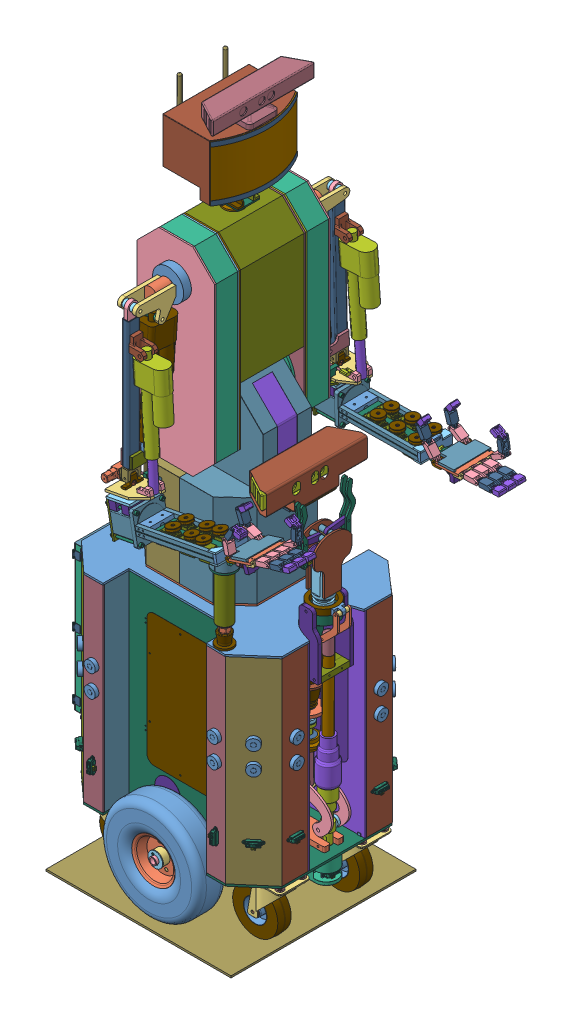
SolidWorks assembly sorbot, configuration По умолчанию. Lengths in mm. (continued)
Mates (geometry in assembly coordinates): (continued)
- Совпадение572: coincident anti-aligned: plane of HS-311 Hitec Standard Servo and Horn-3/HS-311-p2-1 through (120.3857 893.7008 114.0983) normal (-0.185706 0.982605 0); plane of lower.arm.p9-2 through (118.2362 893.2946 122.4974) normal (0.185706 -0.982605 0)
- Совпадение573: coincident anti-aligned: plane of HS-311 Hitec Standard Servo and Horn-2/HS-311-p2-1 through (174.429 903.9147 111.5983) normal (-0.185706 0.982605 0); plane of lower.arm.p9-5 through (172.2795 903.5084 119.9974) normal (0.185706 -0.982605 0)
- Совпадение574: coincident anti-aligned: plane of HS-311 Hitec Standard Servo and Horn-4/HS-311-p2-1 through (203.8531 909.4756 125.8336) normal (-0.185706 0.982605 0); plane of lower.arm.p9-6 through (206.0025 909.8819 117.4346) normal (0.185706 -0.982605 0)
- Заблокировать245: lock: unknown of ?; unknown of lower.arm.p9-4
- Заблокировать246: lock: unknown of ?; unknown of lower.arm.p9-3
- Заблокировать247: lock: unknown of ?; unknown of lower.arm.p9-6
- Заблокировать248: lock: unknown of ?; unknown of lower.arm.p9-5
- Заблокировать249: lock: unknown of ?; unknown of lower.arm.p9-2
- Заблокировать250: lock: unknown of lower.arm.p2-1; unknown of lower.arm.p8-2
- Совпадение582: coincident anti-aligned: plane of palm.p1-3 through (364.9952 940.9838 91.5947) normal (0.311571 -0.950223 0); plane of palm.p3-1 through (346.841 935.0312 91.3484) normal (-0.311571 0.950223 0)
- Совпадение583: coincident anti-aligned: plane of palm.p1-3 through (361.9011 946.2836 191.5864) normal (0.950144 0.311545 0.012888); plane of palm.p3-1 through (362.0352 950.0109 91.5947) normal (-0.950144 -0.311545 -0.012888)
- Совпадение584: coincident aligned: plane of palm.p1-3 through (290.6402 922.9177 190.6197) normal (-0.012247 -0.004016 0.999917); plane of palm.p3-1 through (369.3773 952.4183 191.7026) normal (-0.012247 -0.004016 0.999917)
- Заблокировать261: lock: unknown of lower.arm.p8-2; unknown of palm.fixture.p4-4
- Заблокировать262: lock: unknown of lower.arm.p8-2; unknown of palm.fixture.p4-1
- Заблокировать265: lock: unknown of lower.arm.p8-2; unknown of palm.fixture.p4-3
- Заблокировать266: lock: unknown of lower.arm.p8-2; unknown of palm.fixture.p4-5
- Концентричный332: concentric aligned: cylinder of palm.p3-1 through (367.5649 947.6145 91.6528) axis (-0.012247 -0.004016 0.999917) radius 1.5; cylinder of finger.p1-1 through (366.6096 947.3013 169.6463) axis (-0.012247 -0.004016 0.999917) radius 1.5
- Концентричный333: concentric anti-aligned: cylinder of finger.p1-1 through (366.6096 947.3013 169.6463) axis (-0.012247 -0.004016 0.999917) radius 1.5; cylinder of finger.spring-1 through (366.5011 947.2657 178.5056) axis (0.012247 0.004016 -0.999917) radius 1.9307
- Касательный23: tangent anti-aligned: plane of finger.p1-1 through (351.8589 937.2027 182.1761) normal (0.012247 0.004016 -0.999917); cylinder of finger.spring-1 through (357.2133 941.7472 181.9199) axis (0.950144 0.311545 0.012888) radius 0.34
- Параллельность161: parallel aligned: plane of finger.p1-1 through (363.4168 940.9924 169.5819) normal (-0.950144 -0.311545 -0.012888); plane of finger.spring-1 through (357.2133 941.7472 181.9199) normal (-0.950144 -0.311545 -0.012888)
- Концентричный334: concentric aligned: cylinder of palm.p3-1 through (367.5649 947.6145 91.6528) axis (-0.012247 -0.004016 0.999917) radius 1.5; cylinder of palm.fixture.p13-1 through (367.5656 947.6147 91.5963) axis (-0.012247 -0.004016 0.999917) radius 1.5
- Совпадение627: coincident anti-aligned: plane of palm.p3-1 through (362.243 935.8718 186.5483) normal (0.012247 0.004016 -0.999917); plane of finger.p1-1 through (357.4065 939.0217 186.5017) normal (-0.012247 -0.004016 0.999917)
- Параллельность160: parallel aligned: plane of palm.p1-3 through (363.1257 946.6851 91.5947) normal (-0.311571 0.950223 0); plane of finger.p1-1 through (406.9341 967.89 190.7246) normal (-0.311571 0.950223 0)
- Концентричный339: concentric aligned: cylinder of palm.fixture.p13-1 through (367.5656 947.6147 91.5963) axis (-0.012247 -0.004016 0.999917) radius 1.5; cylinder of finger.p1-2 through (367.5465 947.6085 93.1527) axis (-0.012247 -0.004016 0.999917) radius 1.5
- Концентричный342: concentric aligned: cylinder of palm.fixture.p13-1 through (367.5656 947.6147 91.5963) axis (-0.012247 -0.004016 0.999917) radius 1.5; cylinder of finger.p1-3 through (366.9219 947.4037 144.1484) axis (-0.012247 -0.004016 0.999917) radius 1.5
- Параллельность165: parallel aligned: plane of palm.p1-3 through (363.1257 946.6851 91.5947) normal (-0.311571 0.950223 0); plane of finger.p1-3 through (407.2464 967.9924 165.2267) normal (-0.311571 0.950223 0)
- Совпадение637: coincident anti-aligned: plane of palm.p1-3 through (364.9952 940.9838 91.5947) normal (0.311571 -0.950223 0); plane of palm.p3.m-1 through (323.3155 927.3173 191.0376) normal (-0.311571 0.950223 0)
- Совпадение638: coincident aligned: plane of palm.p1-3 through (290.6402 922.9177 190.6197) normal (-0.012247 -0.004016 0.999917); plane of palm.p3.m-1 through (290.9518 925.1246 190.6324) normal (-0.012247 -0.004016 0.999917)
- Совпадение640: coincident anti-aligned: plane of palm.p3.m-1 through (299.2015 928.9006 190.7486) normal (0.950144 0.311545 0.012888); plane of palm.p1-3 through (300.4356 926.1295 166.7506) normal (-0.950144 -0.311545 -0.012888)
- Совпадение641: coincident anti-aligned: plane of palm.p3-1 through (363.3452 936.2333 96.5558) normal (-0.012247 -0.004016 0.999917); plane of finger.p1-2 through (360.8495 937.3933 96.5299) normal (0.012247 0.004016 -0.999917)
- Концентричный345: concentric aligned: cylinder of palm.fixture.p13-1 through (367.5656 947.6147 91.5963) axis (-0.012247 -0.004016 0.999917) radius 1.5; cylinder of finger.p1-4 through (367.2342 947.5061 118.6505) axis (-0.012247 -0.004016 0.999917) radius 1.5
- Параллельность167: parallel aligned: plane of palm.p1-3 through (363.1257 946.6851 91.5947) normal (-0.311571 0.950223 0); plane of finger.p1-4 through (407.5587 968.0948 139.7288) normal (-0.311571 0.950223 0)
- Совпадение645: coincident anti-aligned: plane of palm.p1-3 through (364.9952 940.9838 91.5947) normal (0.311571 -0.950223 0); plane of palm.p3.m-2 through (324.2768 927.6326 112.5441) normal (-0.311571 0.950223 0)
- Совпадение646: coincident aligned: plane of palm.p1-3 through (291.8649 923.3193 90.628) normal (0.012247 0.004016 -0.999917); plane of palm.p3.m-2 through (292.1765 925.5262 90.6407) normal (0.012247 0.004016 -0.999917)
- Совпадение647: coincident anti-aligned: plane of palm.p3.m-2 through (300.1629 929.2158 112.2551) normal (0.950144 0.311545 0.012888); plane of palm.p1-3 through (301.0725 926.3383 114.7549) normal (-0.950144 -0.311545 -0.012888)
- Заблокировать267: lock: unknown of palm.p3-1; unknown of palm.fixture.p13-1
- Концентричный348: concentric aligned: cylinder of palm.p3.m-1 through (296.5509 922.5164 190.6905) axis (0.012247 0.004016 -0.999917) radius 1.5; cylinder of finger.p1-5 through (296.557 922.5184 190.1906) axis (0.012247 0.004016 -0.999917) radius 1.5
- Совпадение648: coincident anti-aligned: plane of palm.p3.m-1 through (289.0079 911.8586 186.555) normal (0.012247 0.004016 -0.999917); plane of finger.p1-5 through (294.0033 910.6326 186.6113) normal (-0.012247 -0.004016 0.999917)
- Концентричный351: concentric aligned: cylinder of finger.p1-6 through (297.5172 922.8332 111.7971) axis (0.012247 0.004016 -0.999917) radius 1.5; cylinder of palm.p3.m-2 through (297.5123 922.8316 112.197) axis (0.012247 0.004016 -0.999917) radius 1.5
- Концентричный352: concentric aligned: cylinder of finger.p1-1 through (405.2463 959.4437 170.1683) axis (-0.012247 -0.004016 0.999917) radius 1.5; cylinder of finger.p2-7 through (405.2463 959.4437 170.1683) axis (-0.012247 -0.004016 0.999917) radius 1.5
- Совпадение652: coincident anti-aligned: plane of finger.p1-1 through (399.3202 952.7649 186.5702) normal (0.012247 0.004016 -0.999917); plane of finger.p2-7 through (396.174 952.0257 186.5287) normal (-0.012247 -0.004016 0.999917)
- Концентричный354: concentric: cylinder of finger.p3-1 through (466.5916 802.6812 273.0909) axis (-0.001318 0.191299 0.981531) radius 1.5; cylinder of finger.p2-7 through (466.5917 802.6596 272.9801) axis (-0.001318 0.191299 0.981531) radius 1.5
- Совпадение653: coincident: plane of finger.p3-1 through (235.2448 521.1837 179.8569) normal (0.004463 0.000114 0.99999); plane of finger.p2-7 through (237.0318 518.7761 179.8492) normal (-0.004463 -0.000114 -0.99999)
- Концентричный355: concentric aligned: cylinder of finger.p1-3 through (405.5586 959.5461 144.6704) axis (-0.012247 -0.004016 0.999917) radius 1.5; cylinder of finger.p2-8 through (405.5586 959.5461 144.6704) axis (-0.012247 -0.004016 0.999917) radius 1.5
- Совпадение654: coincident anti-aligned: plane of finger.p1-3 through (399.6325 952.8673 161.0724) normal (0.012247 0.004016 -0.999917); plane of finger.p2-8 through (396.6473 951.938 161.0321) normal (-0.012247 -0.004016 0.999917)
- Концентричный356: concentric aligned: cylinder of finger.p1-4 through (405.8709 959.6485 119.1725) axis (-0.012247 -0.004016 0.999917) radius 1.5; cylinder of finger.p2-9 through (405.8709 959.6485 119.1725) axis (-0.012247 -0.004016 0.999917) radius 1.5
- Совпадение655: coincident anti-aligned: plane of finger.p1-4 through (399.9448 952.9697 135.5745) normal (0.012247 0.004016 -0.999917); plane of finger.p2-9 through (396.9974 951.997 135.5345) normal (-0.012247 -0.004016 0.999917)
- Концентричный357: concentric aligned: cylinder of finger.p1-2 through (401.9154 969.0333 93.6596) axis (-0.012247 -0.004016 0.999917) radius 1.5; cylinder of finger.p2-10 through (401.9154 969.0333 93.6596) axis (-0.012247 -0.004016 0.999917) radius 1.5
- Совпадение656: coincident anti-aligned: plane of finger.p1-2 through (397.826 961.1324 110.0792) normal (0.012247 0.004016 -0.999917); plane of finger.p2-10 through (406.346 958.4178 110.1726) normal (-0.012247 -0.004016 0.999917)
- Концентричный358: concentric aligned: cylinder of finger.p3-2 through (401.4238 1008.0295 93.9231) axis (-0.012247 -0.004016 0.999917) radius 1.5; cylinder of finger.p2-10 through (401.4252 1008.0299 93.8102) axis (-0.012247 -0.004016 0.999917) radius 1.5
- Совпадение657: coincident anti-aligned: plane of finger.p3-2 through (412.7357 1007.5295 110.4481) normal (-0.012247 -0.004016 0.999917); plane of finger.p2-10 through (405.8167 1000.5207 110.3352) normal (0.012247 0.004016 -0.999917)
- Концентричный359: concentric aligned: cylinder of finger.p1-5 through (287.6988 962.0409 190.2408) axis (0.012247 0.004016 -0.999917) radius 1.5; cylinder of finger.p2-11 through (287.6988 962.0409 190.2408) axis (0.012247 0.004016 -0.999917) radius 1.5
- Совпадение658: coincident anti-aligned: plane of finger.p1-5 through (284.8951 953.7891 186.173) normal (0.012247 0.004016 -0.999917); plane of finger.p2-11 through (278.3955 955.3292 186.0996) normal (-0.012247 -0.004016 0.999917)
- Концентричный360: concentric aligned: cylinder of finger.p3-5 through (307.9454 995.3702 190.7355) axis (0.012247 0.004016 -0.999917) radius 1.5; cylinder of finger.p2-11 through (307.9467 995.3707 190.6226) axis (0.012247 0.004016 -0.999917) radius 1.5
- Совпадение659: coincident anti-aligned: plane of finger.p3-5 through (298.337 1001.6675 186.5299) normal (-0.012247 -0.004016 0.999917); plane of finger.p2-11 through (300.2563 991.3138 186.5118) normal (0.012247 0.004016 -0.999917)
- Концентричный362: concentric aligned: cylinder of finger.p1-6 through (259.3107 936.2716 111.3831) axis (0.012247 0.004016 -0.999917) radius 1.5; cylinder of finger.p2-12 through (259.3107 936.2716 111.3831) axis (0.012247 0.004016 -0.999917) radius 1.5
- Совпадение661: coincident anti-aligned: plane of finger.p1-6 through (264.8581 929.4858 107.4234) normal (0.012247 0.004016 -0.999917); plane of finger.p2-12 through (259.1122 924.7688 107.3341) normal (-0.012247 -0.004016 0.999917)
- Концентричный363: concentric aligned: cylinder of finger.p3-6 through (195.7839 707.1121 106.7239) axis (-0.004463 -0.000114 -0.99999) radius 1.5; cylinder of finger.p2-12 through (195.7834 707.1121 106.6111) axis (-0.004463 -0.000114 -0.99999) radius 1.5
- Совпадение662: coincident: plane of finger.p3-6 through (190.3026 717.2558 102.6343) normal (0.004463 0.000114 0.99999); plane of finger.p2-12 through (187.0589 706.2794 102.6501) normal (-0.004463 -0.000114 -0.99999)
- Совпадение664: coincident anti-aligned: plane of palm.p3-1 through (373.957 939.7128 161.2051) normal (0.012247 0.004016 -0.999917); plane of finger.p1-3 through (357.7188 939.1241 161.0039) normal (-0.012247 -0.004016 0.999917)
- Совпадение665: coincident anti-aligned: plane of palm.p3-1 through (374.2693 939.8152 135.7072) normal (0.012247 0.004016 -0.999917); plane of finger.p1-4 through (358.0311 939.2265 135.506) normal (-0.012247 -0.004016 0.999917)
- Совпадение666: coincident anti-aligned: plane of palm.p1-3 through (363.1257 946.6851 91.5947) normal (-0.311571 0.950223 0); plane of palm.p5-1 through (330.6828 936.0474 170.4076) normal (0.311571 -0.950223 0)
- Совпадение667: coincident anti-aligned: plane of palm.p1-3 through (363.1257 946.6851 91.5947) normal (-0.311571 0.950223 0); plane of palm.p6-1 through (301.0674 926.3367 156.6492) normal (0.311571 -0.950223 0)
- Совпадение668: coincident anti-aligned: plane of palm.p1-3 through (363.1257 946.6851 91.5947) normal (-0.311571 0.950223 0); plane of palm.p5-2 through (331.3758 936.2746 112.4456) normal (0.311571 -0.950223 0)
- Совпадение669: coincident anti-aligned: plane of palm.p1-3 through (363.1257 946.6851 91.5947) normal (-0.311571 0.950223 0); plane of palm.p6-2 through (301.386 926.4412 124.555) normal (0.311571 -0.950223 0)
- Заблокировать268: lock: unknown of palm.p1-3; unknown of palm.cap-1
- Совпадение692: coincident anti-aligned: plane of arm.p1.m-1 through (-3.763 964.7884 152.9102) normal (1 0 0); plane of forearm.rotate.p12-m-1 through (-3.763 985.2277 154.0338) normal (-1 0 0)
- Параллельность178: parallel aligned: plane of forearm.rotate.p12-m-1 through (-3.763 964.7884 154.0338) normal (0 0 1); plane of arm.p1.m-1 through (-18.263 964.7884 156.4102) normal (0 0 1)
- Заблокировать282: lock: unknown of arm.p1.m-1; unknown of forearm.rotate.p12-m-1
- Концентричный381: concentric aligned: cylinder of finger.p3-3 through (442.6662 971.5314 145.2986) axis (-0.012247 -0.004016 0.999917) radius 1.5; cylinder of finger.p2-8 through (442.6677 971.5319 145.173) axis (-0.012247 -0.004016 0.999917) radius 1.5
- Концентричный382: concentric aligned: cylinder of finger.p3-4 through (442.9206 971.8199 119.5969) axis (-0.012247 -0.004016 0.999917) radius 1.5; cylinder of finger.p2-9 through (442.9196 971.8196 119.6752) axis (-0.012247 -0.004016 0.999917) radius 1.5
- Заблокировать287: lock: unknown of finger.p1-1; unknown of finger.spring-2
- Заблокировать288: lock: unknown of finger.p1-1; unknown of finger1.rod-1
- Заблокировать290: lock: unknown of palm.p1-3; unknown of finger.p1-1
- Заблокировать291: lock: unknown of finger.p1-1; unknown of finger.p2-7
- Заблокировать293: lock: unknown of palm.p1-3; unknown of finger.p1-3
- Заблокировать294: lock: unknown of finger.p1-3; unknown of finger.p2-8
- Заблокировать295: lock: unknown of finger.p3-3; unknown of finger.p2-8
- Заблокировать296: lock: unknown of finger.p1-4; unknown of finger.p2-9
- Заблокировать297: lock: unknown of finger.p3-4; unknown of finger.p2-9
- Заблокировать298: lock: unknown of palm.p1-3; unknown of finger.p1-2
- Заблокировать299: lock: unknown of finger.p1-2; unknown of finger.p2-10
- Заблокировать301: lock: unknown of palm.p1-3; unknown of finger.p1-5
- Заблокировать302: lock: unknown of finger.p1-5; unknown of finger.p2-11
- Заблокировать304: lock: unknown of finger.p3-5; unknown of finger.p2-11
- Заблокировать305: lock: unknown of finger.p1-6; unknown of finger.p2-12
- Заблокировать306: lock: unknown of finger.p3-6; unknown of finger.p2-12
- Заблокировать307: lock: unknown of palm.p1-3; unknown of palm.p6-2
- Заблокировать308: lock: unknown of palm.p1-3; unknown of palm.p6-1
- Заблокировать309: lock: unknown of palm.p1-3; unknown of palm.p5-2
- Заблокировать310: lock: unknown of palm.p1-3; unknown of palm.p5-1
- Заблокировать311: lock: unknown of palm.p1-3; unknown of palm.fixture.p14-1
- Заблокировать319: lock: unknown of palm.p3-1; unknown of palm.fixture.p13-1
- Концентричный386: concentric aligned: cylinder of body.frame.p1-3 through (-12.4559 1335.4922 -50.7442) axis (0 0 1) radius 43; cylinder of arm.fixture.cap-1 through (-12.4559 1335.4922 -73.2442) axis (0 0 1) radius 45
- Заблокировать330: lock: unknown of body_axis-1; unknown of body.frame.p1.fixture-1
- Заблокировать336: lock: unknown of body.frame.p2-1; unknown of body.frame.p1-3
- Заблокировать337: lock: unknown of body.frame.p2-1; unknown of body.frame.p3-1
- Совпадение740: coincident anti-aligned: plane of shoulder.bearing.housing-2 through (-12.4903 1335.516 -46.7442) normal (0 0 1); plane of body.frame.p4.right-1 through (-117.4903 1436.2936 -46.7442) normal (0 0 -1)
- Концентричный404: concentric aligned: cylinder of shoulder.bearing.housing-1 through (-12.7629 1335.3853 40.2558) axis (0 0 -1) radius 15.5; cylinder of shoulder.axis-1 through (-12.7629 1335.3853 44.2558) axis (0 0 -1) radius 15
- Совпадение742: coincident: unknown of shoulder.bearing.housing-2; unknown of shoulder.axis-1
- Заблокировать361: lock: unknown of shoulder.p6-1; unknown of shoulder.axis-1
- Заблокировать362: lock: unknown of shoulder.p6-2; unknown of shoulder.axis-1
- Совпадение745: coincident anti-aligned: plane of body.frame.p5-1 through (92.4017 957.5916 592.5032) normal (1 0 0); plane of cap-hinge-1 through (92.4017 1325.4557 -46.5922) normal (-1 0 0)
- Совпадение746: coincident anti-aligned: plane of body.frame.p5-1 through (92.4017 957.5916 592.5032) normal (1 0 0); plane of cap-hinge-p1-2 through (92.4017 1182.6154 -46.8053) normal (-1 0 0)
- Концентричный405: concentric anti-aligned: cylinder of cap-hinge-2 through (95.4017 1143.4534 -46.8053) axis (0 1 0) radius 2; cylinder of cap-hinge-p1-2 through (95.4017 1182.6154 -46.8053) axis (0 -1 0) radius 2
- Совпадение747: coincident anti-aligned: plane of cap-hinge-2 through (75.4017 1173.4534 -40.9717) normal (0 -1 0); plane of cap-hinge-p1-2 through (75.4017 1173.4534 -41.8622) normal (0 1 0)
- Заблокировать363: lock: unknown of body.frame.p5-1; unknown of cap-hinge-1
- Заблокировать364: lock: unknown of body.frame.p5-1; unknown of cap-hinge-p1-2
- Касательный31: tangent anti-aligned: cylinder of arm.actuator.p2-2 through (-12.7848 967.3083 102.1523) axis (0 0.997661 -0.068351) radius 10; plane of forearm.rotate.p12-1 through (-22.7848 999.7884 125.248) normal (1 0 0)
- Параллельность188: parallel anti-aligned: cylinder of arm.actuator-2/arm.actuator.p1-1 through (-27.7848 1286.6873 80.2712) axis (1 0 0) radius 4.1; cylinder of arm.actuator.p2-2 through (12.2152 975.7884 101.5713) axis (-1 0 0) radius 4
- Заблокировать368: lock: unknown of shoulder.axis-1; unknown of arm.fixture-2
- Заблокировать369: lock: unknown of arm.p1.m-1; unknown of shoulder.lever-1
- Совпадение765: coincident anti-aligned: plane of arm.p1.m-1 through (-18.263 964.7884 125.9102) normal (0 0 1); plane of shoulder.lever-1 through (-17.763 1335.3853 125.9102) normal (0 0 -1)
- Концентричный406: concentric anti-aligned: cylinder of arm.fixture-2 through (-27.7629 1335.3853 140.1602) axis (-1 0 0) radius 4; cylinder of shoulder.lever-1 through (-17.763 1335.3853 140.1602) axis (1 0 0) radius 4
- Концентричный408: concentric aligned: cylinder of arm.lift2.actuator.fixture.p1-1 through (-17.763 1335.3853 140.1602) axis (-1 0 0) radius 4; cylinder of arm.fixture-2 through (-27.7629 1335.3853 140.1602) axis (-1 0 0) radius 4
- Совпадение757: coincident anti-aligned: plane of shoulder.lever-1 through (-17.763 1335.3853 140.1608) normal (-1 0 0); plane of arm.lift2.actuator.fixture.p1-1 through (-17.763 1335.3853 140.1602) normal (1 0 0)
- Концентричный409: concentric anti-aligned: cylinder of arm.actuator-2/arm.actuator.p1-1 through (-27.7848 1286.6873 80.2712) axis (1 0 0) radius 4.1; cylinder of arm.fixture-2 through (-27.7629 1286.6873 80.2712) axis (-1 0 0) radius 4
- Совпадение759: coincident anti-aligned: plane of arm.fixture-2 through (-27.7629 1335.3734 139.2441) normal (1 0 0); plane of arm.lift2.actuator.fixture.p1.m1-1 through (-27.7629 1286.6873 80.2712) normal (-1 0 0)
- Концентричный411: concentric anti-aligned: cylinder of arm.actuator-2/arm.actuator.p1-1 through (-27.7848 1286.6873 80.2712) axis (1 0 0) radius 4.1; cylinder of arm.lift2.actuator.fixture.p1.m1-1 through (-22.7629 1286.6873 80.2712) axis (-1 0 0) radius 4
- Совпадение760: coincident anti-aligned: plane of shoulder.axis-1 through (2.2371 1356.1502 -67.7442) normal (1 0 0); plane of arm.fixture-3 through (2.2371 1335.3734 139.2441) normal (-1 0 0)
- Концентричный412: concentric anti-aligned: cylinder of shoulder.lever-1 through (-17.763 1335.3853 140.1602) axis (1 0 0) radius 4; cylinder of arm.fixture-3 through (12.2371 1335.3853 140.1602) axis (-1 0 0) radius 4
- Концентричный413: concentric aligned: cylinder of arm.fixture-3 through (12.2371 1335.3853 140.1602) axis (-1 0 0) radius 4; cylinder of arm.lift2.actuator.fixture.p1-3 through (2.2371 1335.3853 140.1602) axis (-1 0 0) radius 4
- Совпадение761: coincident anti-aligned: plane of arm.fixture-3 through (2.2371 1335.3734 139.2441) normal (-1 0 0); plane of arm.lift2.actuator.fixture.p1-3 through (2.2371 1335.3853 140.1602) normal (1 0 0)
- Концентричный414: concentric anti-aligned: cylinder of arm.actuator-2/arm.actuator.p1-1 through (-27.7848 1286.6873 80.2712) axis (1 0 0) radius 4.1; cylinder of arm.lift2.actuator.fixture.p1.m1-2 through (2.2371 1286.6873 80.2712) axis (-1 0 0) radius 4
- Совпадение762: coincident anti-aligned: plane of arm.fixture-3 through (2.2371 1335.3734 139.2441) normal (-1 0 0); plane of arm.lift2.actuator.fixture.p1.m1-2 through (2.2371 1286.6873 80.2712) normal (1 0 0)
- Концентричный416: concentric anti-aligned: cylinder of arm.actuator-2/arm.actuator.p1-1 through (-27.7848 1286.6873 80.2712) axis (1 0 0) radius 4.1; cylinder of arm.fixture-3 through (12.2371 1286.6873 80.2712) axis (-1 0 0) radius 4
- Заблокировать370: lock: unknown of shoulder.axis-1; unknown of arm.fixture-3
- Концентричный420: concentric aligned: cylinder of body.center-1 through (-20.0648 982.0246 -136.9555) axis (0 -1 0) radius 11; cylinder of body_pivot-2 through (-20.0648 982.0246 -136.9555) axis (0 -1 0) radius 11
- Заблокировать371: lock: unknown of body.center-1; unknown of body_pivot_fixture-1
- Совпадение768: coincident anti-aligned: plane of body_pivot_fixture-1 through (-20.0648 972.0246 -136.9555) normal (0 1 0); plane of body_pivot-2 through (-63.8424 972.0246 -151.4602) normal (0 -1 0)
- Заблокировать372: lock: unknown of body.frame.p2-1; unknown of cap-hinge-p1-1
- Концентричный421: concentric anti-aligned: cylinder of body_axis-1 through (-20.0648 1016.5246 -50.7475) axis (0 0 -1) radius 10.9; cylinder of body.tilt.axis.frame-2 through (-20.0648 1016.5246 -110.5942) axis (0 0 1) radius 11
- Совпадение776: coincident anti-aligned: plane of body_pivot-2 through (-63.8424 982.0246 -151.4602) normal (0 1 0); plane of body.tilt.axis.frame-2 through (1.9352 982.0246 -116.0942) normal (0 -1 0)
- Концентричный422: concentric aligned: cylinder of body_axis-1 through (-20.0648 1016.5246 -50.7475) axis (0 0 -1) radius 10.9; cylinder of body.tilt.axis.frame-3 through (-20.0648 1016.5246 -163.4875) axis (0 0 -1) radius 11
- Совпадение779: coincident anti-aligned: plane of body_pivot-2 through (-63.8424 982.0246 -151.4602) normal (0 1 0); plane of body.tilt.axis.frame-3 through (1.9352 982.0246 -157.9875) normal (0 -1 0)
- Концентричный430: concentric anti-aligned: cylinder of tilt.thread.rod-1 through (-119.3768 948.5591 -141.6211) axis (0 -1 0) radius 8; cylinder of tilt.thread.rod.fixture.2-1 through (-119.3768 794.5591 -141.6211) axis (0 1 0) radius 8
- Совпадение797: coincident anti-aligned: plane of tilt.thread.rod-1 through (-119.3768 794.5591 -141.6211) normal (0 -1 0); plane of tilt.thread.rod.fixture.2-1 through (-119.3768 794.5591 -141.6211) normal (0 1 0)
- Концентричный431: concentric: cylinder of tilt.thread.rod-1 through (-118.5699 947.5591 -137.5376) axis (0 -1 0) radius 8; cylinder of tilit.thread.rod.bearing.fixture-1 through (-118.5701 937.0246 -137.4966) axis (0 -1 0) radius 6.5
- Совпадение799: coincident anti-aligned: plane of tilit.thread.rod.bearing.fixture-1 through (-20.0648 937.0246 -136.9555) normal (0 1 0); plane of tilit.thread.bearing-1 through (-119.3768 937.0246 -141.6211) normal (0 -1 0)
- Концентричный432: concentric anti-aligned: cylinder of tilt.thread.rod-1 through (-119.3768 928.5591 -141.6211) axis (0 1 0) radius 6; cylinder of tilit.thread.bearing-1 through (-119.3768 945.0246 -141.6211) axis (0 -1 0) radius 6
- Совпадение800: coincident anti-aligned: plane of tilit.thread.rod.bearing.fixture-1 through (-20.0648 937.0246 -136.9555) normal (0 1 0); plane of tilit.thread.rod.bearing.housing-1 through (-119.3768 937.0246 -141.6211) normal (0 -1 0)
- Концентричный433: concentric aligned: cylinder of tilit.thread.bearing-1 through (-119.3768 945.0246 -141.6211) axis (0 -1 0) radius 14; cylinder of tilit.thread.rod.bearing.housing-1 through (-119.3768 945.0246 -141.6211) axis (0 -1 0) radius 14
- Концентричный434: concentric anti-aligned: cylinder of body_axis-1 through (-20.0648 1016.5246 -50.7475) axis (0 0 -1) radius 10.9; cylinder of body_tilt_axis_clamp-1 through (-20.0648 1016.5246 -155.4875) axis (0 0 1) radius 11
- Совпадение801: coincident anti-aligned: plane of body.tilt.axis.frame-3 through (-20.0648 1016.5246 -163.4875) normal (0 0 1); plane of body_tilt_axis_clamp-1 through (-20.0648 1016.5246 -163.4875) normal (0 0 -1)
- Концентричный435: concentric aligned: cylinder of body_axis-1 through (-20.0648 1016.5246 -50.7475) axis (0 0 -1) radius 10.9; cylinder of body_tilt_axis_clamp-2 through (-20.0648 1016.5246 -110.5942) axis (0 0 -1) radius 10.9
- Совпадение802: coincident anti-aligned: plane of body.tilt.axis.frame-2 through (-20.0648 1016.5246 -110.5942) normal (0 0 -1); plane of body_tilt_axis_clamp-2 through (-20.0648 1016.5246 -110.5942) normal (0 0 1)
- Концентричный436: concentric anti-aligned: cylinder of body_tilt_axis_clamp-1 through (-20.0648 1016.5246 -155.4875) axis (0 0 1) radius 20; cylinder of body_tilt_lever-1 through (-20.0648 1016.5246 -149.4875) axis (0 0 -1) radius 20
- Совпадение803: coincident anti-aligned: plane of body_tilt_axis_clamp-1 through (-20.0648 1016.5246 -155.4875) normal (0 0 1); plane of body_tilt_lever-1 through (-97.2168 978.7734 -155.4875) normal (0 0 -1)
- Заблокировать382: lock: unknown of body_pivot-2; unknown of body.tilt.axis.frame-3
- Заблокировать383: lock: unknown of body_pivot-2; unknown of body.tilt.axis.frame-2
- Заблокировать386: lock: unknown of body_axis-1; unknown of body_tilt_axis_clamp-2
- Заблокировать387: lock: unknown of body_axis-1; unknown of body_tilt_axis_clamp-1
- Заблокировать388: lock: unknown of body_pivot_fixture-1; unknown of body_pivot-2
- Заблокировать389: lock: unknown of body_tilt_axis_clamp-1; unknown of body_tilt_lever-1
- Заблокировать391: lock: unknown of body_pivot_fixture-1; unknown of tilit.thread.rod.bearing.fixture-1
- Концентричный439: concentric aligned: cylinder of body_tilt_axis_clamp-2 through (-20.0648 1016.5246 -118.5942) axis (0 0 -1) radius 20; cylinder of body_tilt_lever-2 through (-20.0648 1016.5246 -118.5942) axis (0 0 -1) radius 20
- Концентричный440: concentric aligned: cylinder of body_tilt_lever-1 through (-99.3474 976.856 -149.4875) axis (0 0 -1) radius 5; cylinder of body_tilt_lever-2 through (-99.3474 976.856 -118.5942) axis (0 0 -1) radius 5
- Совпадение805: coincident anti-aligned: plane of body_tilt_axis_clamp-2 through (-20.0648 1016.5246 -118.5942) normal (0 0 -1); plane of body_tilt_lever-2 through (-97.2168 978.7734 -118.5942) normal (0 0 1)
- Концентричный441: concentric aligned: cylinder of body_tilt_lever-1 through (-99.3474 976.856 -149.4875) axis (0 0 -1) radius 5; cylinder of body_tilt_lever_axis-1 through (-99.3474 976.856 -80.4875) axis (0 0 -1) radius 5
- Расстояние22: distance = 40 mm aligned: plane of body_tilt_lever-1 through (-97.2168 978.7734 -155.4875) normal (0 0 -1); plane of body_tilt_lever_axis-1 through (-99.3474 976.856 -195.4875) normal (0 0 -1)
- Концентричный442: concentric anti-aligned: cylinder of body.tilit.lever.2-1 through (-99.3474 976.856 -188.4655) axis (0 0 1) radius 5; cylinder of body_tilt_lever_axis-1 through (-99.3474 976.856 -80.4875) axis (0 0 -1) radius 5
- Концентричный443: concentric anti-aligned: cylinder of tilt.thread.rod-1 through (-119.3768 928.5591 -141.6211) axis (0 1 0) radius 6; cylinder of body.tilt.nut-1 through (-119.3768 842.3995 -141.6211) axis (0 -1 0) radius 8
- Концентричный444: concentric anti-aligned: cylinder of tilt.thread.rod-1 through (-119.3768 928.5591 -141.6211) axis (0 1 0) radius 6; cylinder of body.tilit.nut.housing-1 through (-119.3768 838.3995 -141.6211) axis (0 -1 0) radius 8
- Концентричный445: concentric anti-aligned: cylinder of body.tilit.lever.2-1 through (-119.3768 828.3995 -188.4655) axis (0 0 1) radius 5; cylinder of body.tilit.nut.housing-1 through (-119.3768 828.3995 -156.4655) axis (0 0 -1) radius 5
- Концентричный446: concentric aligned: cylinder of body.tilit.nut.housing-1 through (-119.3768 828.3995 -156.4655) axis (0 0 -1) radius 5; cylinder of body.tilit.nut.housing.bolt-1 through (-119.3768 828.3995 -158.4655) axis (0 0 -1) radius 5
- Совпадение808: coincident anti-aligned: plane of body.tilt.nut-1 through (-110.3768 828.3995 -126.0327) normal (0 -1 0); plane of body.tilit.nut.housing-1 through (-94.3768 828.3995 -157.2211) normal (0 1 0)
- Параллельность198: parallel anti-aligned: plane of body.tilt.nut-1 through (-110.3768 842.3995 -157.2096) normal (0 0 -1); plane of body.tilit.nut.housing-1 through (-144.3768 828.3995 -157.2211) normal (0 0 1)
- Заблокировать392: lock: unknown of body.tilit.nut.housing-1; unknown of body.tilit.nut.housing.cap-1
- Совпадение810: coincident anti-aligned: plane of body.tilit.lever.2-1 through (-119.3768 828.3995 -181.4655) normal (0 0 1); plane of body.tilit.nut.housing-1 through (-141.3638 838.3995 -181.4655) normal (0 0 -1)
- Совпадение811: coincident anti-aligned: plane of body.tilit.lever.2-1 through (-119.3768 828.3995 -188.4655) normal (0 0 -1); plane of body.tilit.nut.housing.bolt-1 through (-129.642 830.0202 -188.4655) normal (0 0 1)
- Концентричный447: concentric anti-aligned: cylinder of body_tilt_lever_axis-1 through (-99.3474 976.856 -80.4875) axis (0 0 -1) radius 5; cylinder of body.tilit.extender-1 through (-99.3474 976.856 -176.9875) axis (0 0 1) radius 5
- Совпадение812: coincident anti-aligned: plane of body_tilt_lever-1 through (-97.2168 978.7734 -155.4875) normal (0 0 -1); plane of body.tilit.extender-1 through (-99.3474 976.856 -155.4875) normal (0 0 1)
- Концентричный448: concentric aligned: cylinder of body_tilt_lever_axis-1 through (-99.3474 976.856 -80.4875) axis (0 0 -1) radius 5; cylinder of washer-1 through (-99.3474 976.856 -188.4655) axis (0 0 -1) radius 5
- Совпадение813: coincident anti-aligned: plane of body.tilit.lever.2-1 through (-119.3768 828.3995 -188.4655) normal (0 0 -1); plane of washer-1 through (-99.3474 976.856 -188.4655) normal (0 0 1)
- Концентричный449: concentric anti-aligned: cylinder of body_tilt_lever_axis-1 through (-99.3474 976.856 -80.4875) axis (0 0 -1) radius 5; cylinder of body.tilit.extender-2 through (-99.3474 976.856 -118.5942) axis (0 0 1) radius 5
- Совпадение814: coincident anti-aligned: plane of body_tilt_lever-2 through (-97.2168 978.7734 -118.5942) normal (0 0 1); plane of body.tilit.extender-2 through (-99.3474 976.856 -118.5942) normal (0 0 -1)
- Концентричный450: concentric anti-aligned: cylinder of body_tilt_lever_axis-1 through (-99.3474 976.856 -80.4875) axis (0 0 -1) radius 5; cylinder of body.tilit.lever.2-2 through (-99.3474 976.856 -101.7768) axis (0 0 1) radius 5
- Концентричный451: concentric aligned: cylinder of body.tilit.nut.housing-1 through (-119.3768 828.3995 -126.7768) axis (0 0 1) radius 5; cylinder of body.tilit.lever.2-2 through (-119.3768 828.3995 -101.7768) axis (0 0 1) radius 5
- Совпадение816: coincident anti-aligned: plane of body.tilit.nut.housing-1 through (-141.3638 838.3995 -101.7768) normal (0 0 1); plane of body.tilit.lever.2-2 through (-119.3768 828.3995 -101.7768) normal (0 0 -1)
- Концентричный452: concentric aligned: cylinder of body.tilit.nut.housing-1 through (-119.3768 828.3995 -126.7768) axis (0 0 1) radius 5; cylinder of body.tilit.nut.housing.bolt-2 through (-119.3768 828.3995 -124.7768) axis (0 0 1) radius 5
- Совпадение817: coincident anti-aligned: plane of body.tilit.lever.2-2 through (-119.3768 828.3995 -94.7768) normal (0 0 1); plane of body.tilit.nut.housing.bolt-2 through (-109.1117 830.0202 -94.7768) normal (0 0 -1)
- Концентричный453: concentric aligned: cylinder of body_tilt_lever_axis-1 through (-99.3474 976.856 -80.4875) axis (0 0 -1) radius 5; cylinder of washer-2 through (-99.3474 976.856 -92.7768) axis (0 0 -1) radius 5
- Совпадение818: coincident anti-aligned: plane of body.tilit.lever.2-2 through (-119.3768 828.3995 -94.7768) normal (0 0 1); plane of washer-2 through (-99.3474 976.856 -94.7768) normal (0 0 -1)
- Совпадение819: coincident anti-aligned: plane of body.frame.p1-3 through (92.5097 1436.2936 -50.7442) normal (0 0 -1); plane of arm.fixture.cap-1 through (-12.4559 1335.4922 -50.7442) normal (0 0 1)
- Совпадение820: coincident anti-aligned: plane of finger.p3-2 through (412.7357 1007.5295 110.4481) normal (-0.012247 -0.004016 0.999917); plane of finger.p2-10 through (405.8167 1000.5207 110.3352) normal (0.012247 0.004016 -0.999917)
- Заблокировать394: lock: unknown of finger.p3-2; unknown of finger.p2-10
- Заблокировать395: lock: unknown of finger.p3-1; unknown of finger.p2-7
- Заблокировать396: lock: unknown of body.frame.p1-3; unknown of body.tilit.enforcement-1
- Заблокировать397: lock: unknown of body.frame.p1.fixture-1; unknown of body.tilit.enforcement-1
- Заблокировать398: lock: unknown of arm.fixture-2; unknown of arm.lift2.actuator.fixture.p1-1
- Заблокировать399: lock: unknown of body.frame.p1.fixture-2; unknown of body.tilit.enforcement-2
- Заблокировать402: lock: unknown of body.frame.p4-4; unknown of body.frame.p5-2
- Заблокировать405: lock: unknown of body.frame.p2-1; unknown of cap-hinge-4
- Концентричный459: concentric anti-aligned: cylinder of cap-hinge-p1-3 through (95.5097 1327.1115 -226.3787) axis (0 -1 0) radius 2; cylinder of cap-hinge-5 through (95.5097 1287.9494 -226.3787) axis (0 1 0) radius 2
- Совпадение845: coincident anti-aligned: plane of cap-hinge-p1-3 through (75.5097 1317.9494 -221.4356) normal (0 1 0); plane of cap-hinge-5 through (75.5404 1317.9494 -220.4411) normal (0 -1 0)
- Заблокировать404: lock: unknown of body.frame.p2-1; unknown of cap-hinge-p1-3
- Заблокировать406: lock: unknown of body.frame.p5-2; unknown of cap-hinge-5
- Концентричный460: concentric anti-aligned: cylinder of cap-hinge-p1-4 through (95.5097 1143.936 -226.3787) axis (0 1 0) radius 2; cylinder of cap-hinge-4 through (95.5097 1183.1735 -226.3787) axis (0 -1 0) radius 2
- Совпадение847: coincident anti-aligned: plane of cap-hinge-4 through (75.5097 1173.1735 -232.2123) normal (0 -1 0); plane of cap-hinge-p1-4 through (75.4842 1173.1735 -231.2174) normal (0 1 0)
- Заблокировать407: lock: unknown of body.frame.p5-2; unknown of cap-hinge-p1-4
- Заблокировать410: lock: unknown of palm.p3.m-2; unknown of finger.p1-6
- Совпадение849: coincident anti-aligned: plane of body_pivot_fixture-1 through (-20.0648 937.0246 -136.9555) normal (0 -1 0); plane of tilit.thread.rod.bearing.fixture-1 through (-20.0648 937.0246 -136.9555) normal (0 1 0)
- Заблокировать411: lock: unknown of body_pivot_fixture-1; unknown of tilit.thread.rod.bearing.fixture-1
- Заблокировать412: lock: unknown of arm.lift2.actuator.fixture.p1-3; unknown of arm.fixture-3
- Совпадение851: coincident anti-aligned: plane of body.frame.p4-4 through (-117.3772 1436.2936 -226.3595) normal (0 0 1); plane of shoulder.bearing.housing-4 through (-12.3772 1335.516 -226.3595) normal (0 0 -1)
- Концентричный462: concentric aligned: cylinder of body.frame.p4-4 through (-12.3772 1335.516 -226.3595) axis (0 0 -1) radius 12.5; cylinder of shoulder.bearing.housing-4 through (-12.3772 1335.516 -205.3595) axis (0 0 -1) radius 15.5
- Заблокировать413: lock: unknown of body.frame.p4-4; unknown of shoulder.bearing.housing-4
- Концентричный463: concentric aligned: cylinder of shoulder.bearing.housing-3 through (-12.6499 1335.3853 -313.3595) axis (0 0 1) radius 15.5; cylinder of shoulder.axis-2 through (-12.6499 1335.3853 -317.3595) axis (0 0 1) radius 15
- Совпадение853: coincident aligned: plane of shoulder.bearing.housing-4 through (-12.3772 1335.516 -205.3595) normal (0 0 1); plane of shoulder.axis-2 through (-12.6499 1335.3853 -205.3595) normal (0 0 1)
- Совпадение855: coincident: plane of body.frame.p4-4 through (-117.3772 1436.2936 -230.3595) normal (0 0 -1); unknown of shoulder.p6-3
- Совпадение856: coincident anti-aligned: plane of shoulder.p6-4 through (-12.6499 1335.3853 -288.3595) normal (0 0 -1); plane of body.frame.p4.external-1 through (-117.6384 1436.1749 -288.3595) normal (0 0 1)
- Концентричный464: concentric aligned: cylinder of shoulder.axis-2 through (-12.6499 1335.3853 -317.3595) axis (0 0 1) radius 15; cylinder of shoulder.p6-3 through (-12.6499 1335.3853 -245.2739) axis (0 0 1) radius 15
- Концентричный465: concentric anti-aligned: cylinder of shoulder.axis-2 through (-12.6499 1335.3853 -317.3595) axis (0 0 1) radius 15; cylinder of shoulder.p6-4 through (-12.6499 1335.3853 -270.3595) axis (0 0 -1) radius 15
- Совпадение857: coincident: unknown of shoulder.p6-3; plane of shoulder.p4-3 through (-59.8188 1400.1357 -245.3595) normal (0 0 1)
- Совпадение858: coincident anti-aligned: plane of shoulder.p6-4 through (-12.6499 1335.3853 -270.3595) normal (0 0 1); plane of shoulder.p4-4 through (-59.8188 1400.1357 -270.3595) normal (0 0 -1)
- Концентричный466: concentric anti-aligned: cylinder of shoulder.axis-2 through (-12.6499 1335.3853 -317.3595) axis (0 0 1) radius 15; cylinder of shoulder.p4-4 through (-12.6499 1335.3853 -266.3595) axis (0 0 -1) radius 15
- Концентричный467: concentric anti-aligned: cylinder of shoulder.axis-2 through (-12.6499 1335.3853 -317.3595) axis (0 0 1) radius 15; cylinder of shoulder.p4-3 through (-12.6499 1335.3853 -245.3595) axis (0 0 -1) radius 15
- Совпадение865: coincident anti-aligned: plane of body.frame.p4-4 through (-117.3772 1436.2936 -230.3595) normal (0 0 -1); plane of arm.lift.actuator.fixture.p3-3 through (-88.5702 993.1387 -230.3595) normal (0 0 1)
- Концентричный469: concentric aligned: cylinder of arm.lift.actuator.fixture.p3-3 through (-88.5702 993.1387 -230.3595) axis (0 0 -1) radius 4; cylinder of arm.lift.actuator.fixture.p2-2 through (-88.5702 993.1387 -230.3595) axis (0 0 -1) radius 4
- Заблокировать416: lock: unknown of arm.lift.actuator.fixture.p3-3; unknown of arm.lift.actuator.fixture.p2-2
- Заблокировать415: lock: unknown of body.frame.p4-4; unknown of arm.lift.actuator.fixture.p3-3
- Концентричный470: concentric anti-aligned: cylinder of arm.lift.actuator.fixture.p3-4 through (-88.5702 993.1387 -288.3595) axis (0 0 1) radius 4; cylinder of arm.lift.actuator.fixture.p2-2 through (-88.5702 993.1387 -230.3595) axis (0 0 -1) radius 4
- Концентричный478: concentric aligned: cylinder of arm.lift.actuator.fixture.p2-2 through (-88.5702 993.1387 -230.3595) axis (0 0 -1) radius 4; cylinder of arm.actuator-4/arm.actuator.p1-1 through (-88.5702 993.1387 -244.3595) axis (0 0 -1) radius 4.1
- Касательный33: tangent anti-aligned: plane of arm.lift.actuator.fixture.p3-3 through (-88.5702 993.1387 -249.3595) normal (0 0 -1); cylinder of arm.actuator-4/arm.actuator.p1-1 through (-89.1112 985.157 -259.3595) axis (0.067628 0.997711 0) radius 10
- Концентричный480: concentric anti-aligned: cylinder of arm.actuator-4/arm.actuator.p1-1 through (-79.508 1126.8319 -259.3595) axis (0.067628 0.997711 0) radius 10; cylinder of arm.actuator.p2-4 through (-60.3086 1410.0778 -259.3595) axis (-0.067628 -0.997711 0) radius 10
- Концентричный482: concentric anti-aligned: cylinder of shoulder.p4-4 through (-60.8835 1401.5972 -266.3595) axis (0 0 -1) radius 4; cylinder of arm.actuator.p2-4 through (-60.8835 1401.5972 -284.3595) axis (0 0 1) radius 4
- Концентричный481: concentric anti-aligned: cylinder of shoulder.p4-3 through (-60.8835 1401.5972 -245.3595) axis (0 0 -1) radius 4; cylinder of arm.actuator.p2-4 through (-60.8835 1401.5972 -284.3595) axis (0 0 1) radius 4
- Заблокировать418: lock: unknown of shoulder.axis-2; unknown of arm.fixture-4
- Заблокировать419: lock: unknown of shoulder.axis-2; unknown of arm.fixture-5
- Концентричный483: concentric anti-aligned: cylinder of arm.fixture-4 through (2.8485 1335.3868 -413.2628) axis (0.999986 0 0.005196) radius 4; cylinder of arm.lift2.actuator.fixture.p1-4 through (2.8485 1335.3868 -413.2628) axis (-0.999986 0 -0.005196) radius 4
- Совпадение869: coincident anti-aligned: plane of arm.fixture-4 through (2.8437 1335.375 -412.3468) normal (-0.999986 0 -0.005196); plane of arm.lift2.actuator.fixture.p1-4 through (2.8485 1335.3868 -413.2628) normal (0.999986 0 0.005196)
- Заблокировать420: lock: unknown of arm.fixture-4; unknown of arm.lift2.actuator.fixture.p1-4
- Концентричный484: concentric aligned: cylinder of shoulder.lever-2 through (-7.1514 1335.3868 -413.3148) axis (-0.999986 0 -0.005196) radius 4; cylinder of arm.lift2.actuator.fixture.p1-4 through (2.8485 1335.3868 -413.2628) axis (-0.999986 0 -0.005196) radius 4
- Совпадение870: coincident anti-aligned: plane of shoulder.lever-2 through (-7.1514 1335.3868 -413.3154) normal (0.999986 0 0.005196); plane of arm.lift2.actuator.fixture.p1-4 through (-7.1514 1335.3868 -413.3148) normal (-0.999986 0 -0.005196)
- Концентричный485: concentric anti-aligned: cylinder of arm.fixture-5 through (-37.1514 1335.3868 -413.3148) axis (0.999986 0 0.005196) radius 4; cylinder of arm.lift2.actuator.fixture.p1-5 through (-17.1517 1335.3868 -413.2109) axis (-0.999986 0 -0.005196) radius 4
- Совпадение871: coincident anti-aligned: plane of arm.fixture-5 through (-27.1563 1335.375 -412.3468) normal (0.999986 0 0.005196); plane of arm.lift2.actuator.fixture.p1-5 through (-27.1515 1335.3868 -413.2628) normal (-0.999986 0 -0.005196)
- Заблокировать422: lock: unknown of shoulder.lever-2; unknown of arm.p1.m-2
- Концентричный486: concentric anti-aligned: cylinder of arm.fixture-4 through (2.5373 1286.6879 -353.3754) axis (0.999986 0 0.005196) radius 4; cylinder of arm.actuator-5/arm.actuator.p1-1 through (2.5373 1286.6879 -353.3754) axis (-0.999986 0 -0.005196) radius 4.1
- Концентричный487: concentric anti-aligned: cylinder of arm.fixture-4 through (2.5373 1286.6879 -353.3754) axis (0.999986 0 0.005196) radius 4; cylinder of arm.lift2.actuator.fixture.p1.m1-3 through (2.5373 1286.6879 -353.3754) axis (-0.999986 0 -0.005196) radius 4
- Совпадение873: coincident anti-aligned: plane of arm.fixture-4 through (2.8437 1335.375 -412.3468) normal (-0.999986 0 -0.005196); plane of arm.lift2.actuator.fixture.p1.m1-3 through (2.5373 1286.6879 -353.3754) normal (0.999986 0 0.005196)
- Концентричный488: concentric anti-aligned: cylinder of arm.fixture-5 through (-37.4626 1286.6879 -353.4274) axis (0.999986 0 0.005196) radius 4; cylinder of arm.lift2.actuator.fixture.p1.m1-4 through (-22.4628 1286.6879 -353.3495) axis (-0.999986 0 -0.005196) radius 4
- Совпадение874: coincident anti-aligned: plane of arm.fixture-5 through (-27.1563 1335.375 -412.3468) normal (0.999986 0 0.005196); plane of arm.lift2.actuator.fixture.p1.m1-4 through (-27.4627 1286.6879 -353.3754) normal (-0.999986 0 -0.005196)
- Касательный34: tangent anti-aligned: cylinder of arm.actuator-5/arm.actuator.p1-1 through (-12.4664 1294.6528 -352.7052) axis (0.000486 -0.995617 -0.093518) radius 10; plane of arm.lift2.actuator.fixture.p1.m1-3 through (-2.4627 1286.6879 -353.4014) normal (-0.999986 0 -0.005196)
- Заблокировать423: lock: unknown of shoulder.p6-3; unknown of shoulder.p4-3
- Заблокировать424: lock: unknown of shoulder.p6-4; unknown of shoulder.p4-4
- Заблокировать425: lock: unknown of shoulder.axis-2; unknown of shoulder.p6-3
- Заблокировать426: lock: unknown of shoulder.axis-2; unknown of shoulder.p6-4
- Заблокировать427: lock: unknown of arm.p1.m-2; unknown of forearm.rotate.p12-m-2
- Заблокировать428: lock: unknown of arm.p1.m-2; unknown of forearm.rotate.p12-2
- Заблокировать429: lock: unknown of arm.p1.m-2; unknown of forearm.rotate.p9-2
- Заблокировать430: lock: unknown of arm.p1.m-2; unknown of actuator.100.fixture-2
- Концентричный493: concentric aligned: cylinder of actuator.100.fixture-2 through (30.5425 1248.8767 -435.037) axis (-0.005195 -0.022106 0.999742) radius 4; cylinder of arm.actuator100mm..p1-2 through (30.516 1248.7636 -429.924) axis (-0.005195 -0.022106 0.999742) radius 4
- Касательный35: tangent anti-aligned: plane of actuator.100.fixture-2 through (40.8098 1209.6631 -405.7286) normal (0.005195 0.022106 -0.999742); cylinder of arm.actuator100mm..p1-2 through (29.9802 1256.417 -414.7536) axis (0.057231 -0.998124 -0.021773) radius 10
- Концентричный495: concentric anti-aligned: cylinder of arm.actuator100mm..p1-2 through (35.3599 1162.5934 -416.8003) axis (0.057231 -0.998124 -0.021773) radius 10; cylinder of arm.actuator100mm.p2-2 through (49.2611 920.154 -422.0889) axis (-0.057231 0.998124 0.021773) radius 10
- Заблокировать445: lock: unknown of lower.arm.p2-5; unknown of lower.arm.p8-3
- Заблокировать446: lock: unknown of lower.arm.p3-2; unknown of ?
- Заблокировать447: lock: unknown of lower.arm.p3-2; unknown of ?
- Заблокировать448: lock: unknown of lower.arm.p3-2; unknown of ?
- Заблокировать449: lock: unknown of lower.arm.p3-2; unknown of ?
- Заблокировать450: lock: unknown of lower.arm.p3-2; unknown of ?
- Заблокировать451: lock: unknown of lower.arm.p3-2; unknown of ?
- Концентричный504: concentric anti-aligned: cylinder of HS-311 Hitec Standard Servo and Horn-12/HS-311-p2-1 through (110.806 865.1228 -440.1318) axis (-0.012385 0.99968 0.022041) radius 4.064; cylinder of lower.arm.p9-8 through (110.7286 871.3708 -439.994) axis (0.012385 -0.99968 -0.022041) radius 12
- Концентричный505: concentric anti-aligned: cylinder of HS-311 Hitec Standard Servo and Horn-8/HS-311-p2-1 through (165.824 865.856 -442.4703) axis (-0.012385 0.99968 0.022041) radius 4.064; cylinder of lower.arm.p9-10 through (165.7466 872.104 -442.3326) axis (0.012385 -0.99968 -0.022041) radius 12
- Концентричный506: concentric anti-aligned: cylinder of HS-311 Hitec Standard Servo and Horn-10/HS-311-p2-1 through (220.8415 866.5874 -444.7289) axis (-0.012385 0.99968 0.022041) radius 4.064; cylinder of lower.arm.p9-12 through (220.7641 872.8354 -444.5912) axis (0.012385 -0.99968 -0.022041) radius 12
- Концентричный507: concentric anti-aligned: cylinder of HS-311 Hitec Standard Servo and Horn-11/HS-311-p2-1 through (110.6228 864.3429 -404.8609) axis (-0.012385 0.99968 0.022041) radius 4.064; cylinder of lower.arm.p9-7 through (110.5453 870.5909 -404.7231) axis (0.012385 -0.99968 -0.022041) radius 12
- Концентричный508: concentric anti-aligned: cylinder of HS-311 Hitec Standard Servo and Horn-7/HS-311-p2-1 through (165.6133 864.9593 -401.9208) axis (-0.012385 0.99968 0.022041) radius 4.064; cylinder of lower.arm.p9-9 through (165.5359 871.2073 -401.783) axis (0.012385 -0.99968 -0.022041) radius 12
